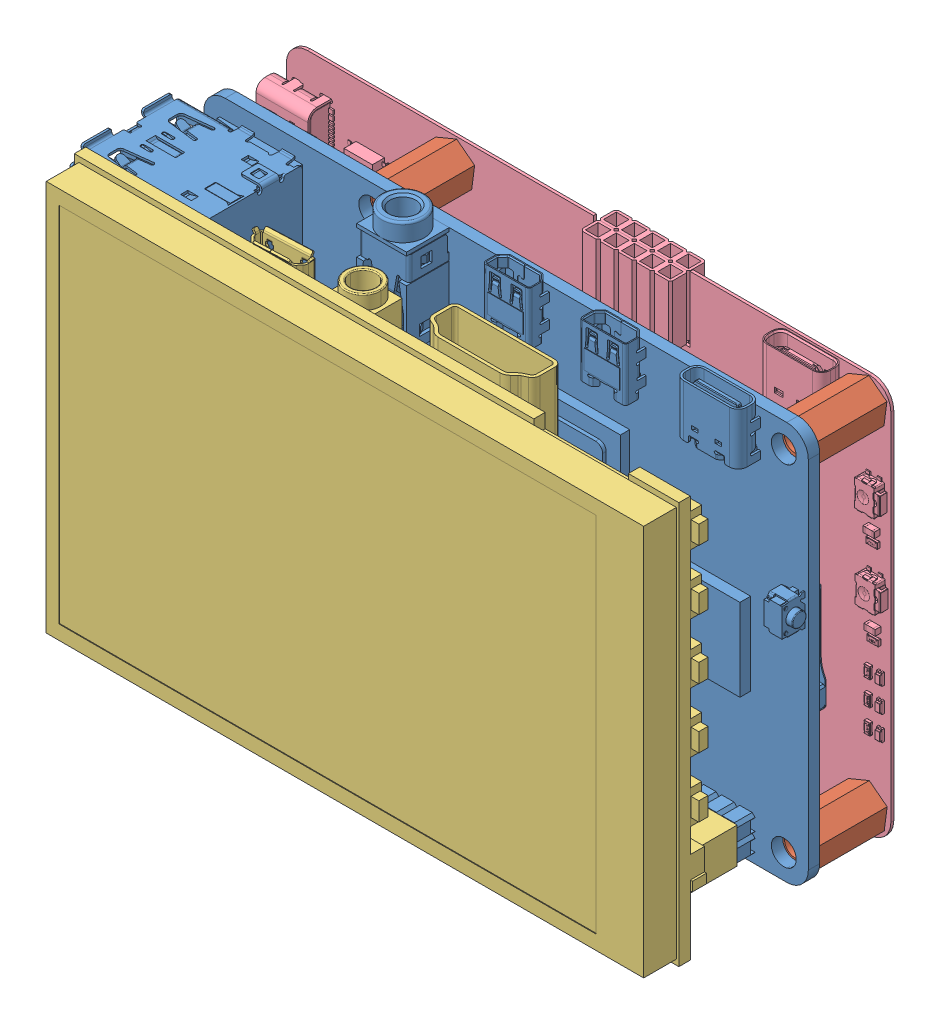
SolidWorks assembly 处理单元, configuration 默认. Lengths in mm.
Overall size (88.74 58.85 36.44).
7 component instances, 4 part files, 12 mates.
Components (placement in the parent):
- ROCK4CP-1: ROCK4CP [默认] at (-24.6274 5.4497 104.0605) x (0 -1 0) z (0 0 1) size (58.5 88.56 19.4)
- M3-10mm铜柱-1: M3-10mm铜柱 [默认] at (-43.8721 29.8762 92.4605) x (-0.923728 -0.383049 0) z (-0.383049 0.923728 0) size (6.35 10 5.5)
- M3-10mm铜柱-2: M3-10mm铜柱 [默认] at (-43.8721 -19.2238 92.4605) x (-0.923728 -0.383049 0) z (-0.383049 0.923728 0) size (6.35 10 5.5)
- M3-10mm铜柱-3: M3-10mm铜柱 [默认] at (14.1279 -19.2238 92.4605) x (-0.923728 -0.383049 0) z (-0.383049 0.923728 0) size (6.35 10 5.5)
- M3-10mm铜柱-4: M3-10mm铜柱 [默认] at (14.0903 30.084 92.4605) x (-0.923728 -0.383049 0) z (-0.383049 0.923728 0) size (6.35 10 5.5)
- 3.5寸屏幕-1: 3.5寸屏幕 [默认] at (-25.3265 5.3488 123.1605) x (-1 0 0) z (0 0 -1) size (86 57.54 19.6)
- 核心板载板-V1-2: 核心板载板-V1 [默认] at (-67.1265 -22.5493 92.4605) size (86.13 56 8.72)
Mates (geometry in assembly coordinates):
- 同心5: concentric anti-aligned: circle of ROCK4CP-1; circle of M3-10mm铜柱-2
- 重合5: coincident anti-aligned: plane of ROCK4CP-1 through (-24.6274 5.4497 102.4605) normal (0 0 -1); plane of M3-10mm铜柱-2 through (-43.8721 -19.2238 102.4605) normal (0 0 1)
- 同心8: concentric anti-aligned: circle of ROCK4CP-1; circle of M3-10mm铜柱-3
- 重合6: coincident anti-aligned: plane of ROCK4CP-1 through (9.1035 -20.2812 106.5605) normal (0 0 1); plane of 3.5寸屏幕-1 through (-25.3265 -29.1658 106.5605) normal (0 0 -1)
- 重合7: coincident aligned: plane of ROCK4CP-1 through (7.4335 -21.5512 106.5605) normal (0 -1 0); plane of 3.5寸屏幕-1 through (10.3735 -21.5512 119.9605) normal (0 -1 0)
- 重合8: coincident aligned: plane of ROCK4CP-1 through (10.3735 -21.1512 106.5605) normal (1 0 0); plane of 3.5寸屏幕-1 through (10.3735 -16.5512 119.9605) normal (1 0 0)
- 重合10: coincident aligned: circle of M3-10mm铜柱-1; plane of 核心板载板-V1-2 through (-67.1265 -19.5493 92.4605) normal (0 0 1)
- 重合11: coincident aligned: plane of ROCK4CP-1 through (17.8735 -19.5524 104.0605) normal (1 0 0); plane of 核心板载板-V1-2 through (17.8735 30.4507 92.049) normal (1 0 0)
- 重合14: coincident aligned: plane of ROCK4CP-1 through (14.8401 33.4507 104.0605) normal (0 1 0); plane of 核心板载板-V1-2 through (-10.3575 33.4507 92.049) normal (0 1 0)
- 重合16: coincident anti-aligned: plane of M3-10mm铜柱-4 through (14.0903 30.084 92.4605) normal (0 0 -1); plane of 核心板载板-V1-2 through (-67.1265 -19.5493 92.4605) normal (0 0 1)
- 重合17: coincident anti-aligned: plane of ROCK4CP-1 through (-24.6274 5.4497 102.4605) normal (0 0 -1); plane of M3-10mm铜柱-4 through (14.0903 30.084 102.4605) normal (0 0 1)
- 重合18: coincident anti-aligned: plane of ROCK4CP-1 through (-24.6274 5.4497 102.4605) normal (0 0 -1); plane of M3-10mm铜柱-3 through (14.1279 -19.2238 102.4605) normal (0 0 1)
